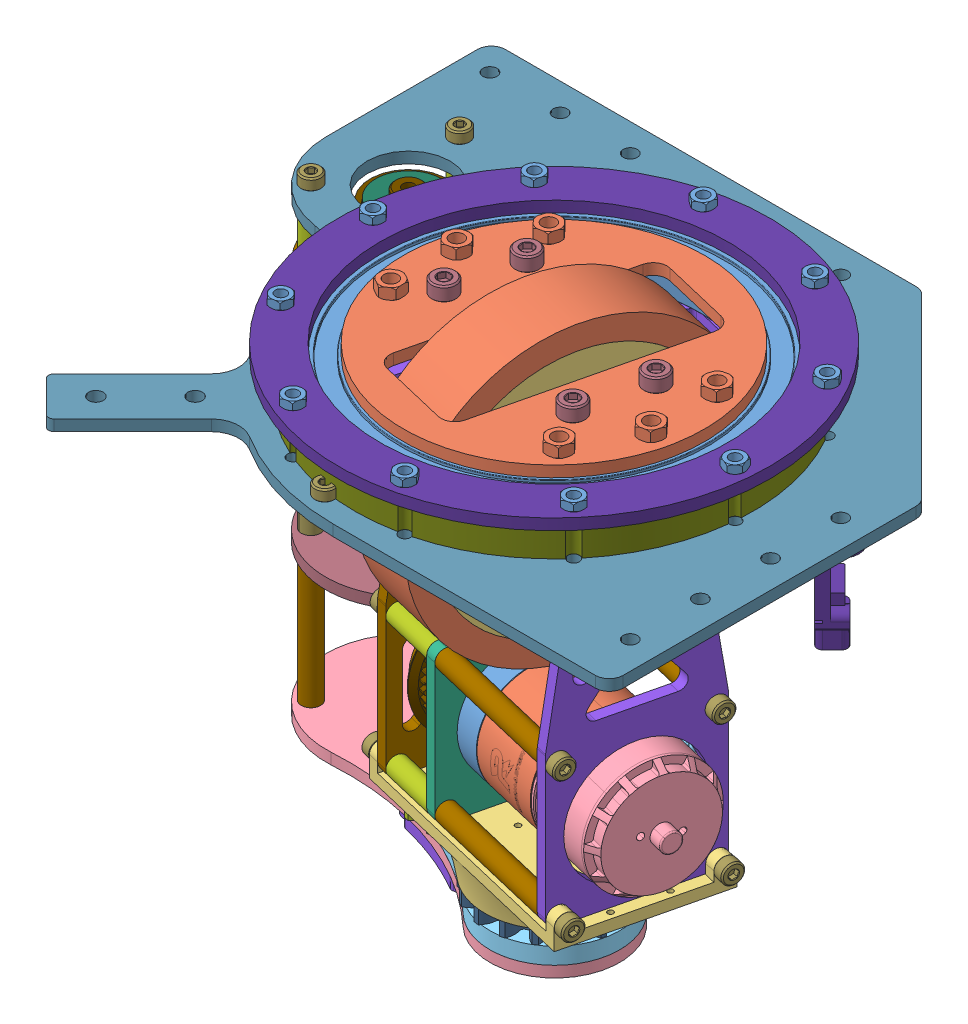
SolidWorks assembly 舵轮装配3508转向板R, configuration 默认. Lengths in mm.
Overall size (849.08 223.15 204.82).
168 component instances, 59 part files, 248 mates.
Components (placement in the parent):
- am-0198 4in Plaction Wheel-1: am-0198 4in Plaction Wheel [默认] at (-7.6128 -124.2866 103.0773) x (0.972741 0 0.231893) z (0.060048 0.965891 -0.25189)
  - am-0198 4in Plaction Wheel(2)^am-0198 4in Plaction Wheel-1: am-0198 4in Plaction Wheel(2)^am-0198 4in Plaction Wheel [默认] at origin (virtual)
- HRB 61821薄圈轴承-1: HRB 61821薄圈轴承 [默认] at (-20.3948 -93.8434 93.3472) x (0.952416 0 0.304802) z (-0.304802 0 0.952416) size (130 13 130)
- 舵轮底板-1: 舵轮底板 [默认] at (-20.3948 -80.8434 93.3472) x (0.231893 0 -0.972741) z (0.972741 0 0.231893) size (109 4 109)
- 舵轮侧面支撑-1: 舵轮侧面支撑 [默认] at (8.3011 -80.8434 100.1881) x (-0.972741 0 -0.231893) z (-0.231893 0 0.972741) size (14 45 35)
- 22 8 7轴承-1: 22 8 7轴承 [默认] at (-15.0447 -115.8434 94.6227) x (-0.972741 0 -0.231893) z (0.221934 -0.28991 -0.930966) size (7 25 25)
- 舵轮用钢轴-1: 舵轮用钢轴 [默认] at (13.1648 -115.8434 101.3476) x (-0.0855 0.929546 0.358656) z (-0.215555 -0.368706 0.904208) size (8 70 8)
- 舵轮侧面支撑B-1: 舵轮侧面支撑B [默认] at (-52.9816 -80.8434 85.5788) x (0.972741 0 0.231893) z (0.231893 0 -0.972741) size (8 45 35)
- 舵轮轴承契合垫-1: 舵轮轴承契合垫 [默认] at (-20.3948 -93.8434 93.3472) x (-0.972741 0 -0.231893) z (0.231893 0 -0.972741) size (18.69 13 65.65)
- 舵轮上底板-1: 舵轮上底板 [默认] at (-20.3948 -97.8434 93.3472) x (0.231893 0 -0.972741) z (0.972741 0 0.231893) size (120 4 120)
- M3508电机安装板-1: M3508电机安装板 [默认] at (-56.8726 -93.3434 84.6513) x (0 1 0) z (-0.231893 0 0.972741) size (145.98 4 55)
- RoboMaster M3508直流无刷减速电-1: RoboMaster M3508直流无刷减速电 [默认] at (54.6807 -194.7601 92.9675) x (0.079289 -0.939729 -0.332601) z (-0.972741 0 -0.231893) size (77.46 77.46 98.4)
  - RoboMaster M3508直流无刷减速电 (1).STEP-1: RoboMaster M3508直流无刷减速电 (1).STEP [默认] at origin size (77.46 77.46 98.4)
    - 4_ASM_1.STEP-1: 4_ASM_1.STEP [默认] at (-1.7887 18.2683 39.841) x (-0.923508 0.383579 0) z (0.383579 0.923508 0) size (13.16 4.26 21.29)
      - __-__10_1__1.STEP-1: __-__10_1__1.STEP [默认] at origin size (2.4 2.3 2.24)
      - __-__10_3__1.STEP-1: __-__10_3__1.STEP [默认] at origin size (2.4 2.3 2.24)
      - __-__10_2__1.STEP-1: __-__10_2__1.STEP [默认] at origin size (2.4 2.3 2.24)
      - __-__20_1.STEP-1: __-__20_1.STEP [默认] at origin size (5.92 4.26 12.18)
    - 2_ASM.STEP-1: 2_ASM.STEP [默认] at (-1.7887 18.2683 50.441) x (-0.378508 0.925598 0) z (0.925598 0.378508 0) size (59.4 67.29 59.4)
      - 26_ASM.STEP-1: 26_ASM.STEP [默认] at (0 34.5 0) x (-0.381788 0 0.92425) z (-0.92425 0 -0.381788) size (22 6 22)
        - 28_1.STEP-1: 28_1.STEP [默认] at (0 2.5 0) size (20 0.2 20)
        - 27_1.STEP-1: 27_1.STEP [默认] at origin size (22 6 22)
        - 28_1.STEP-2: 28_1.STEP [默认] at (0 -2.7 0) size (20 0.2 20)
      - 26_ASM-1.STEP-1: 26_ASM-1.STEP [默认] at (0 27 0) x (-0.381788 0 0.92425) z (-0.92425 0 -0.381788) size (22 6 22)
        - 28_1.STEP-1: 28_1.STEP [默认] at (0 2.5 0) size (20 0.2 20)
        - 27_1.STEP-1: 27_1.STEP [默认] at origin size (22 6 22)
        - 28_1.STEP-2: 28_1.STEP [默认] at (0 -2.7 0) size (20 0.2 20)
      - 25_1.STEP-1: 25_1.STEP [默认] at (0 38.5 0) x (0 0 1) z (-1 0 0) size (16.7 1 13.43)
      - 18_1.STEP-1: 18_1.STEP [默认] at (-12.3744 22 -12.3744) x (0.381788 0 -0.92425) z (0.92425 0 0.381788) size (5.5 37.99 5.5)
      - 17_1.STEP-1: 17_1.STEP [默认] at (0 19.3 0) x (-1 0 0) z (0 0 -1) size (26 44 26)
      - 16_1.STEP-1: 16_1.STEP [默认] at (0 31 0) x (-0.707107 0 0.707107) z (0 1 0) size (42 42 14)
      - 18_1.STEP-2: 18_1.STEP [默认] at (12.3744 22 -12.3744) x (0.92425 0 0.381788) z (-0.381788 0 0.92425) size (5.5 37.99 5.5)
      - 23_1.STEP-1: 23_1.STEP [默认] at origin size (42.11 26 42)
      - 18_1.STEP-3: 18_1.STEP [默认] at (12.3744 22 12.3744) x (-0.381788 0 0.92425) z (-0.92425 0 -0.381788) size (5.5 37.99 5.5)
      - 18_1.STEP-4: 18_1.STEP [默认] at (-12.3744 22 12.3744) x (-0.92425 0 -0.381788) z (0.381788 0 -0.92425) size (5.5 37.99 5.5)
      - 24_1.STEP-1: 24_1.STEP [默认] at (0 37.71 0) x (0 1 0) z (0.381788 0 -0.92425) size (0.42 16 16)
    - 1_1_1.STEP-1: 1_1_1.STEP [默认] at (-1.7887 18.2683 48.441) x (0.923508 -0.383579 0) z (0 0 1) size (42 42 43.4)
    - 3_1.STEP-1: 3_1.STEP [默认] at (4.5067 -1.7659 43.091) x (0.299781 -0.954008 0) z (0.954008 0.299781 0) size (5.77 4 14.5)
- M3508电机安装延长-1: M3508电机安装延长 [默认] at (-37.4178 -199.3254 89.2891) x (0 1 0) z (0.231893 0 -0.972741) size (55 4 55)
- 螺纹M4_长度20铝柱-1: 螺纹M4_长度20铝柱 [默认] at (-42.9832 -223.3254 112.6349) x (0.178665 -0.637485 -0.749461) z (0.147828 0.770463 -0.620108) size (7 20 7)
- 螺纹M4_长度20铝柱-2: 螺纹M4_长度20铝柱 [默认] at (-31.8523 -223.3254 65.9433) x (0.178665 -0.637485 -0.749461) z (0.147828 0.770463 -0.620108) size (7 20 7)
- 螺纹M4_长度20铝柱-3: 螺纹M4_长度20铝柱 [默认] at (-42.9832 -175.3254 112.6349) x (0.178665 -0.637485 -0.749461) z (0.147828 0.770463 -0.620108) size (7 20 7)
- 螺纹M4_长度20铝柱-4: 螺纹M4_长度20铝柱 [默认] at (-31.8523 -175.3254 65.9433) x (0.178665 -0.637485 -0.749461) z (0.147828 0.770463 -0.620108) size (7 20 7)
- M3508电机安装板B-1: M3508电机安装板B [默认] at (19.0012 -93.3434 102.7389) x (0 1 0) z (-0.231893 0 0.972741) size (145.98 4 55)
- 螺纹M4_长度50铝柱-1: 螺纹M4_长度50铝柱 [默认] at (20.6757 -175.3254 78.4655) x (0.131851 -0.822624 -0.553086) z (0.190761 0.568585 -0.800201) size (7 50 7)
- 螺纹M4_长度50铝柱-2: 螺纹M4_长度50铝柱 [默认] at (20.6757 -223.3254 78.4655) x (0.131851 -0.822624 -0.553086) z (0.190761 0.568585 -0.800201) size (7 50 7)
- 螺纹M4_长度50铝柱-3: 螺纹M4_长度50铝柱 [默认] at (9.5448 -223.3254 125.1571) x (0.131851 -0.822624 -0.553086) z (0.190761 0.568585 -0.800201) size (7 50 7)
- 螺纹M4_长度50铝柱-4: 螺纹M4_长度50铝柱 [默认] at (9.5448 -175.3254 125.1571) x (0.131851 -0.822624 -0.553086) z (0.190761 0.568585 -0.800201) size (7 50 7)
- 舵轮用100齿3m同步带-1: 舵轮用100齿3m同步带 [默认] at (-39.6585 -199.3254 88.7549) x (-0.00142 0.999981 0.005957) z (-0.231889 -0.006124 0.972723) size (119.08 7 42.19)
- 舵轮轴承契合垫B-1: 舵轮轴承契合垫B [默认] at (-20.3948 -93.8434 93.3472) x (0.972741 0 0.231893) z (-0.231893 0 0.972741) size (18.69 13 65.65)
- M4螺丝头-3: M4螺丝头 [默认] at (-66.329 -175.3254 107.0695) x (0.075861 -0.944977 -0.31822) z (0.219133 0.327137 -0.919218) size (7.2 4.15 7.2)
- M4螺丝头-4: M4螺丝头 [默认] at (-55.1981 -175.3254 60.3779) x (0.077323 -0.94277 -0.324353) z (0.218622 0.333443 -0.917072) size (7.2 4.15 7.2)
- M4螺丝头-6: M4螺丝头 [默认] at (24.5667 -175.3254 79.3931) x (0.143947 0.784011 -0.603826) z (0.181807 -0.620747 -0.76264) size (7.2 4.15 7.2)
- M4螺丝头-7: M4螺丝头 [默认] at (13.4358 -175.3254 126.0847) x (0.143947 0.784011 -0.603826) z (0.181807 -0.620747 -0.76264) size (7.2 4.15 7.2)
- M5螺丝头-1: M5螺丝头 [默认] at (17.8418 -85.8434 107.6026) x (0.144633 0.781658 -0.606706) z (0.181261 -0.623708 -0.760351) size (8.7 5.42 8.7)
- M5螺丝头-2: M5螺丝头 [默认] at (20.1607 -85.8434 97.8752) x (0.144633 0.781658 -0.606706) z (0.181261 -0.623708 -0.760351) size (8.7 5.42 8.7)
- M5螺丝头-3: M5螺丝头 [默认] at (21.3202 -100.8434 93.0115) x (0.143947 0.784011 -0.603826) z (0.181807 -0.620747 -0.76264) size (8.7 5.42 8.7)
- M5螺丝头-4: M5螺丝头 [默认] at (16.6823 -100.8434 112.4663) x (0.143947 0.784011 -0.603826) z (0.181807 -0.620747 -0.76264) size (8.7 5.42 8.7)
- 舵轮转向同步轮 75齿-3: 舵轮转向同步轮 75齿 [默认] at (-20.4563 -110.3434 93.5041) x (0.231893 0 -0.972741) z (0 1 0) size (120.22 120.22 12.5)
- 螺纹M4_长度20铝柱-5: 螺纹M4_长度20铝柱 [默认] at (-118.8835 -117.8434 29.0349) x (0.334336 0 -0.942454) z (0.942454 0 0.334336) size (7 20 7)
- 螺纹M4_长度20铝柱-6: 螺纹M4_长度20铝柱 [默认] at (-131.2035 -117.8434 70.5466) x (0.991825 0 0.127608) z (-0.127608 0 0.991825) size (7 20 7)
- 螺纹M4_长度20铝柱-7: 螺纹M4_长度20铝柱 [默认] at (-89.0934 -117.8434 60.4602) x (0.952416 0 0.304802) z (-0.304802 0 0.952416) size (7 20 7)
- 舵轮转向驱动同步轮15齿-1: 舵轮转向驱动同步轮15齿 [默认] at (-113.0601 -108.8434 53.3472) x (0.894911 0 0.446244) z (0 1 0) size (23.73 23.73 12)
- M5螺丝头-7: M5螺丝头 [默认] at (25.1276 -105.3434 79.7838) x (-0.621955 0 -0.783053) z (-0.783053 0 0.621955) size (8.7 5.42 8.7)
- M5螺丝头-8: M5螺丝头 [默认] at (25.8104 -105.3434 104.3622) x (-0.598714 0 -0.800963) z (-0.800963 0 0.598714) size (8.7 5.42 8.7)
- M5螺丝头-9: M5螺丝头 [默认] at (14.1126 -105.3434 125.989) x (-0.602334 0 -0.798244) z (-0.798244 0 0.602334) size (8.7 5.42 8.7)
- M5螺丝头-10: M5螺丝头 [默认] at (-54.9022 -105.3434 60.7054) x (-0.578379 0 -0.815768) z (-0.815768 0 0.578379) size (8.7 5.42 8.7)
- M5螺丝头-11: M5螺丝头 [默认] at (-66.6 -105.3434 82.3323) x (-0.630623 0 -0.776089) z (-0.776089 0 0.630623) size (8.7 5.42 8.7)
- M5螺丝头-12: M5螺丝头 [默认] at (-58.4446 -100.8434 73.9963) x (0.084545 -0.931169 -0.35465) z (0.215931 0.364588 -0.905786) size (8.7 5.42 8.7)
- M5螺丝头-13: M5螺丝头 [默认] at (-65.9171 -105.3434 106.9107) x (-0.636639 0 -0.771162) z (-0.771162 0 0.636639) size (8.7 5.42 8.7)
- M5螺丝头-14: M5螺丝头 [默认] at (-63.0825 -100.8434 93.4511) x (0.110669 -0.878771 -0.464234) z (0.203781 0.477243 -0.854817) size (8.7 5.42 8.7)
- 舵轮大轴承定位环-1: 舵轮大轴承定位环 [默认] at (-20.3948 -93.8434 93.3472) x (0.224951 0 0.97437) z (-0.97437 0 0.224951) size (144.14 13 144.2)
- 轴承压住-1: 轴承压住 [默认] at (-20.3948 -80.8434 93.3472) x (-0.390731 0 0.920505) z (-0.920505 0 -0.390731) size (156 4 156)
- 舵轮转向同步带90齿5m-1: 舵轮转向同步带90齿5m [默认] at (-113.0601 -108.8434 53.3472) x (-0.394392 0 0.918942) z (-0.918942 0 -0.394392) size (124.22 10 176.93)
- M4螺丝头-15: M4螺丝头 [默认] at (-74.8093 -97.8434 46.0454) x (-0.630623 0 -0.776089) z (-0.776089 0 0.630623) size (7.2 4.15 7.2)
- M4螺丝头-16: M4螺丝头 [默认] at (-36.6138 -97.8434 23.0952) x (-0.630623 0 -0.776089) z (-0.776089 0 0.630623) size (7.2 4.15 7.2)
- M4螺丝头-17: M4螺丝头 [默认] at (7.7769 -97.8434 26.9788) x (-0.630623 0 -0.776089) z (-0.776089 0 0.630623) size (7.2 4.15 7.2)
- M4螺丝头-18: M4螺丝头 [默认] at (41.407 -97.8434 56.213) x (-0.630623 0 -0.776089) z (-0.776089 0 0.630623) size (7.2 4.15 7.2)
- M4螺丝头-19: M4螺丝头 [默认] at (51.4309 -97.8434 99.6312) x (-0.630623 0 -0.776089) z (-0.776089 0 0.630623) size (7.2 4.15 7.2)
- M4螺丝头-20: M4螺丝头 [默认] at (34.0198 -97.8434 140.6491) x (-0.630623 0 -0.776089) z (-0.776089 0 0.630623) size (7.2 4.15 7.2)
- M4螺丝头-21: M4螺丝头 [默认] at (-4.1758 -97.8434 163.5993) x (-0.630623 0 -0.776089) z (-0.776089 0 0.630623) size (7.2 4.15 7.2)
- M4螺丝头-22: M4螺丝头 [默认] at (-48.5665 -97.8434 159.7156) x (-0.630623 0 -0.776089) z (-0.776089 0 0.630623) size (7.2 4.15 7.2)
- M4螺丝头-23: M4螺丝头 [默认] at (-82.1965 -97.8434 130.4815) x (-0.630623 0 -0.776089) z (-0.776089 0 0.630623) size (7.2 4.15 7.2)
- M4螺丝头-24: M4螺丝头 [默认] at (-92.2204 -97.8434 87.0633) x (-0.630623 0 -0.776089) z (-0.776089 0 0.630623) size (7.2 4.15 7.2)
- M4螺母-1: M4螺母 [默认] at (51.4309 -76.8434 99.6312) x (0.695285 0 0.718734) z (-0.718734 0 0.695285) size (6.78 3.05 7.83)
- M4螺母-3: M4螺母 [默认] at (-4.1758 -76.8434 163.5993) x (0.912983 0 0.407998) z (-0.407998 0 0.912983) size (6.78 3.05 7.83)
- M4螺母-4: M4螺母 [默认] at (-48.5665 -76.8434 159.7156) x (0.955617 0 0.294613) z (-0.294613 0 0.955617) size (6.78 3.05 7.83)
- M4螺母-5: M4螺母 [默认] at (-82.1965 -76.8434 130.4815) x (0.953713 0 0.300718) z (-0.300718 0 0.953713) size (6.78 3.05 7.83)
- M4螺母-6: M4螺母 [默认] at (-92.2204 -76.8434 87.0633) x (0.952416 0 0.304802) z (-0.304802 0 0.952416) size (6.78 3.05 7.83)
- M4螺母-7: M4螺母 [默认] at (-74.8093 -76.8434 46.0454) x (0.952416 0 0.304802) z (-0.304802 0 0.952416) size (6.78 3.05 7.83)
- M4螺母-8: M4螺母 [默认] at (-36.6138 -76.8434 23.0952) x (0.996847 0 0.079344) z (-0.079344 0 0.996847) size (6.78 3.05 7.83)
- M4螺母-9: M4螺母 [默认] at (7.7769 -76.8434 26.9788) x (0.952416 0 0.304802) z (-0.304802 0 0.952416) size (6.78 3.05 7.83)
- M4螺母-10: M4螺母 [默认] at (41.407 -76.8434 56.213) x (0.897027 0 0.441976) z (-0.441976 0 0.897027) size (6.78 3.05 7.83)
- M4螺母-11: M4螺母 [默认] at (34.0198 -76.8434 140.6491) x (0.965082 0 0.261948) z (-0.261948 0 0.965082) size (6.78 3.05 7.83)
- M5螺丝头-15: M5螺丝头 [默认] at (-50.083 -76.8434 73.4196) x (0.952416 0 0.304802) z (-0.304802 0 0.952416) size (8.7 5.42 8.7)
- M5螺丝头-16: M5螺丝头 [默认] at (-55.8803 -76.8434 97.7381) size (8.7 5.42 8.7)
- M5螺丝头-17: M5螺丝头 [默认] at (5.4024 -76.8434 112.3474) x (0.952416 0 0.304802) z (-0.304802 0 0.952416) size (8.7 5.42 8.7)
- M5螺丝头-18: M5螺丝头 [默认] at (11.1997 -76.8434 88.0288) x (0.952416 0 0.304802) z (-0.304802 0 0.952416) size (8.7 5.42 8.7)
- M4螺丝头-25: M4螺丝头 [默认] at (-131.2035 -93.8434 70.5466) x (0.95084 0 0.309681) z (-0.309681 0 0.95084) size (7.2 4.15 7.2)
- M4螺丝头-26: M4螺丝头 [默认] at (-118.8835 -93.8434 29.0349) x (0.952251 0 0.305316) z (-0.305316 0 0.952251) size (7.2 4.15 7.2)
- M4螺丝头-27: M4螺丝头 [默认] at (-31.1775 -93.8434 165.6069) x (0.999978 0 -0.006592) z (0.006592 0 0.999978) size (7.2 4.15 7.2)
- M5螺母-1: M5螺母 [默认] at (14.1126 -76.8434 125.989) x (0.952416 0 0.304802) z (-0.304802 0 0.952416) size (8 4 9.24)
- M5螺母-2: M5螺母 [默认] at (25.8104 -76.8434 104.3622) x (0.952416 0 0.304802) z (-0.304802 0 0.952416) size (8 4 9.24)
- M5螺母-3: M5螺母 [默认] at (25.1276 -76.8434 79.7838) x (0.952416 0 0.304802) z (-0.304802 0 0.952416) size (8 4 9.24)
- M5螺母-4: M5螺母 [默认] at (-54.9022 -76.8434 60.7054) x (0.952416 0 0.304802) z (-0.304802 0 0.952416) size (8 4 9.24)
- M5螺母-5: M5螺母 [默认] at (-66.6 -76.8434 82.3323) x (0.952416 0 0.304802) z (-0.304802 0 0.952416) size (8 4 9.24)
- M5螺母-6: M5螺母 [默认] at (-65.9171 -76.8434 106.9107) x (0.999422 0 -0.034008) z (0.034008 0 0.999422) size (8 4 9.24)
- 舵轮线引导和角度定位3D打印件-1: 舵轮线引导和角度定位3D打印件 [默认] at (-20.7352 -226.8254 93.2661) x (0.231893 0 -0.972741) z (-0.972741 0 -0.231893) size (73.09 24 90.3)
- 理线和舵轮角度定位支撑-1: 理线和舵轮角度定位支撑 [默认] at (-113.0601 -259.8434 53.3472) x (-0.393621 0 0.919273) z (-0.919273 0 -0.393621) size (60 4 154.24)
- 舵轮角度定位第二齿轮轴承锁定-1: 舵轮角度定位第二齿轮轴承锁定 [默认] at (-61.8199 -249.8434 75.2877) x (-0.919273 0 -0.393621) z (0.393621 0 -0.919273) size (93.42 10.62 47)
- 6704zz轴承-1: 6704zz轴承 [默认] at (-61.8199 -253.8434 75.2877) x (0.929857 0 0.36792) z (-0.36792 0 0.929857) size (27 4 27)
- 舵轮角度定位第二齿轮-1: 舵轮角度定位第二齿轮 [默认] at (-61.8199 -247.3434 75.2877) x (0.291333 0 0.956622) z (0 1 0) size (50.24 50.45 15.5)
- M4螺丝头-28: M4螺丝头 [默认] at (-89.0934 -259.8434 60.4602) x (-0.60814 0 -0.79383) z (-0.79383 0 0.60814) size (7.2 4.15 7.2)
- M4螺丝头-30: M4螺丝头 [默认] at (-131.2035 -259.8434 70.5466) x (-0.602759 0 -0.797923) z (-0.797923 0 0.602759) size (7.2 4.15 7.2)
- M4螺丝头-31: M4螺丝头 [默认] at (17.6186 -223.3254 127.0818) x (0.163039 -0.711114 -0.683912) z (-0.164902 -0.703077 0.69173) size (7.2 4.15 7.2)
- M4螺丝头-32: M4螺丝头 [默认] at (-59.0891 -223.3254 59.4503) x (-0.195604 -0.537113 0.820517) z (0.124553 -0.84351 -0.522472) size (7.2 4.15 7.2)
- M4螺丝头-33: M4螺丝头 [默认] at (-70.2199 -223.3254 106.1419) x (0.230329 0.115959 -0.966179) z (-0.02689 0.993254 0.112798) size (7.2 4.15 7.2)
- M4螺丝头-34: M4螺丝头 [默认] at (28.7495 -223.3254 80.3903) x (0.163039 -0.711114 -0.683912) z (-0.164902 -0.703077 0.69173) size (7.2 4.15 7.2)
- 舵轮角度定位AS5600支撑-1: 舵轮角度定位AS5600支撑 [默认] at (-61.8199 -259.8434 75.2877) x (-0.919273 0 -0.393621) z (0.393621 0 -0.919273) size (49.84 4 35.05)
- 舵轮转向电机安装件M3508版本-1: 舵轮转向电机安装件M3508版本 [默认] at (-113.0601 -121.8434 53.3472) x (-0.284517 0 0.958671) z (-0.958671 0 -0.284517) size (60 4 60)
- RoboMaster M3508直流无刷减速电-2: RoboMaster M3508直流无刷减速电 [默认] at (-121.3423 -208.2844 36.9663) x (-0.932142 0 0.362092) z (0 1 0) size (77.46 77.46 98.4)
  - RoboMaster M3508直流无刷减速电 (1).STEP-1: RoboMaster M3508直流无刷减速电 (1).STEP [默认] at origin size (77.46 77.46 98.4)
    - 4_ASM_1.STEP-1: 4_ASM_1.STEP [默认] at (-1.7887 18.2683 39.841) x (-0.923508 0.383579 0) z (0.383579 0.923508 0) size (13.16 4.26 21.29)
      - __-__10_1__1.STEP-1: __-__10_1__1.STEP [默认] at origin size (2.4 2.3 2.24)
      - __-__10_3__1.STEP-1: __-__10_3__1.STEP [默认] at origin size (2.4 2.3 2.24)
      - __-__10_2__1.STEP-1: __-__10_2__1.STEP [默认] at origin size (2.4 2.3 2.24)
      - __-__20_1.STEP-1: __-__20_1.STEP [默认] at origin size (5.92 4.26 12.18)
    - 2_ASM.STEP-1: 2_ASM.STEP [默认] at (-1.7887 18.2683 50.441) x (-0.378508 0.925598 0) z (0.925598 0.378508 0) size (59.4 67.29 59.4)
      - 26_ASM.STEP-1: 26_ASM.STEP [默认] at (0 34.5 0) x (-0.381788 0 0.92425) z (-0.92425 0 -0.381788) size (22 6 22)
        - 28_1.STEP-1: 28_1.STEP [默认] at (0 2.5 0) size (20 0.2 20)
        - 27_1.STEP-1: 27_1.STEP [默认] at origin size (22 6 22)
        - 28_1.STEP-2: 28_1.STEP [默认] at (0 -2.7 0) size (20 0.2 20)
      - 26_ASM-1.STEP-1: 26_ASM-1.STEP [默认] at (0 27 0) x (-0.381788 0 0.92425) z (-0.92425 0 -0.381788) size (22 6 22)
        - 28_1.STEP-1: 28_1.STEP [默认] at (0 2.5 0) size (20 0.2 20)
        - 27_1.STEP-1: 27_1.STEP [默认] at origin size (22 6 22)
        - 28_1.STEP-2: 28_1.STEP [默认] at (0 -2.7 0) size (20 0.2 20)
      - 25_1.STEP-1: 25_1.STEP [默认] at (0 38.5 0) x (0 0 1) z (-1 0 0) size (16.7 1 13.43)
      - 18_1.STEP-1: 18_1.STEP [默认] at (-12.3744 22 -12.3744) x (0.381788 0 -0.92425) z (0.92425 0 0.381788) size (5.5 37.99 5.5)
      - 17_1.STEP-1: 17_1.STEP [默认] at (0 19.3 0) x (-1 0 0) z (0 0 -1) size (26 44 26)
      - 16_1.STEP-1: 16_1.STEP [默认] at (0 31 0) x (-0.707107 0 0.707107) z (0 1 0) size (42 42 14)
      - 18_1.STEP-2: 18_1.STEP [默认] at (12.3744 22 -12.3744) x (0.92425 0 0.381788) z (-0.381788 0 0.92425) size (5.5 37.99 5.5)
      - 23_1.STEP-1: 23_1.STEP [默认] at origin size (42.11 26 42)
      - 18_1.STEP-3: 18_1.STEP [默认] at (12.3744 22 12.3744) x (-0.381788 0 0.92425) z (-0.92425 0 -0.381788) size (5.5 37.99 5.5)
      - 18_1.STEP-4: 18_1.STEP [默认] at (-12.3744 22 12.3744) x (-0.92425 0 -0.381788) z (0.381788 0 -0.92425) size (5.5 37.99 5.5)
      - 24_1.STEP-1: 24_1.STEP [默认] at (0 37.71 0) x (0 1 0) z (0.381788 0 -0.92425) size (0.42 16 16)
    - 1_1_1.STEP-1: 1_1_1.STEP [默认] at (-1.7887 18.2683 48.441) x (0.923508 -0.383579 0) z (0 0 1) size (42 42 43.4)
    - 3_1.STEP-1: 3_1.STEP [默认] at (4.5067 -1.7659 43.091) x (0.299781 -0.954008 0) z (0.954008 0.299781 0) size (5.77 4 14.5)
- 舵轮转向齿轮拼接-1: 舵轮转向齿轮拼接 [默认] at (-20.7352 -248.8254 93.2661) x (-0.972741 0 -0.231893) z (0.231893 0 -0.972741) size (49.13 17 49.32)
- 27_20_4轴承-1: 27_20_4轴承 [默认] at (-20.4526 -255.8434 93.0006) x (0.977214 0 0.212256) z (-0.212256 0 0.977214) size (27 4 27)
- 螺纹M4_长度80铝柱-4: 螺纹M4_长度80铝柱 [默认] at (-118.8835 -201.8434 29.0349) x (-0.231145 0 0.972919) z (-0.972919 0 -0.231145) size (7 80 7)
- 螺纹M4_长度80铝柱-5: 螺纹M4_长度80铝柱 [默认] at (-131.2035 -201.8434 70.5466) x (-0.277096 0 0.960842) z (-0.960842 0 -0.277096) size (7 80 7)
- 螺纹M4_长度80铝柱-6: 螺纹M4_长度80铝柱 [默认] at (-89.0934 -201.8434 60.4602) x (0.668866 0 0.743383) z (-0.743383 0 0.668866) size (7 80 7)
- 舵轮转向电机安装件-3: 舵轮转向电机安装件 [默认] at (-113.0601 -205.8434 53.3472) x (-0.284517 0 0.958671) z (-0.958671 0 -0.284517) size (60 4 60)
- 螺纹M4_长度50铝柱-8: 螺纹M4_长度50铝柱 [默认] at (-131.2035 -255.8434 70.5466) x (0.823062 0 0.567952) z (-0.567952 0 0.823062) size (7 50 7)
- 螺纹M4_长度50铝柱-9: 螺纹M4_长度50铝柱 [默认] at (-118.8835 -255.8434 29.0349) x (0.96384 0 0.266482) z (-0.266482 0 0.96384) size (7 50 7)
- 螺纹M4_长度50铝柱-10: 螺纹M4_长度50铝柱 [默认] at (-89.0934 -255.8434 60.4602) x (0.841404 0 -0.540407) z (0.540407 0 0.841404) size (7 50 7)
- 舵轮直角安装架R-1: 舵轮直角安装架R [默认] at (-285.7255 -97.8434 93.3472) size (222.67 4 198.17)
- as5600安装架小-1: as5600安装架小 [默认] at (-61.8199 -261.8434 75.2877) x (0.393621 0 -0.919273) z (-0.919273 0 -0.393621) size (23 3 23)
- 第二齿轮上固定-1: 第二齿轮上固定 [默认] at (-61.8199 -251.8434 75.2877) x (-0.956622 0 0.291333) z (0.291333 0 0.956622) size (22 3.5 22)
- as5600安装架小-2: as5600安装架小 [默认] at (-61.8199 -267.8434 75.2877) x (0.919273 0 0.393621) z (-0.393621 0 0.919273) size (23 3 23)
- 配电板支架R-1: 配电板支架R [默认] at (31.5052 -97.8434 41.4472) x (0 0 -1) z (-1 0 0) size (89.5 55 843.45)
- 40齿3M同步轮-1: 40齿3M同步轮 [GearTrax] at (-50.3552 -199.3254 86.2049) x (0.009093 0.999231 -0.038144) z (0.972741 0 0.231893) size (43.17 43.17 18.61)
- 16_8_5轴承-1: 16_8_5轴承 [默认] at (-27.5931 -115.8434 91.6312) x (0.972741 0 0.231893) z (-0.231392 0.065672 0.970641) size (5 17 17)
- 包胶轮子装配-1: 包胶轮子装配 [默认] at (-7.0413 -25.7462 40.883) x (0.20398 -0.475659 -0.855652) z (-0.110302 -0.87963 0.462693) size (105 25 105)
  - 定制轮子包胶部分-1: 定制轮子包胶部分 [默认] at (-4.7594 -13.3234 105) size (105 25 105)
  - 定制轮子铝合金部分-1: 定制轮子铝合金部分 [默认] at (-4.7594 -13.3234 105) size (88 25 88)
- 包胶轮子同步轮-1: 包胶轮子同步轮 [默认] at (-57.0824 24.1318 171.778) x (0.20398 -0.475659 -0.855652) z (0.972741 0 0.231893) size (63 58.51 16)
- 包胶轮子垫圈-1: 包胶轮子垫圈 [默认] at (1.4919 -115.8434 98.5648) x (-0.074139 0.947515 0.310996) z (-0.219722 -0.319711 0.921687) size (20 10 20)
Mates (geometry in assembly coordinates):
- 同心2: concentric aligned: cylinder of HRB 61821薄圈轴承-1 through (-20.3948 -80.8434 93.3472) axis (0 -1 0) radius 65; cylinder of 舵轮底板-1 through (-20.3948 -76.8434 93.3472) axis (0 -1 0) radius 54.5
- 平行1: parallel anti-aligned: plane of am-0198 4in Plaction Wheel-1/am-0198 4in Plaction Wheel(2)^am-0198 4in Plaction Wheel-1/4 Modular Half^am-0198 4in Plaction Wheel(2)_am-0198 4in Plaction Wheel-1 through (-41.2853 -84.2812 91.9114) normal (-0.972741 0 -0.231893); plane of 舵轮底板-1 through (-47.2732 -80.8434 130.6306) normal (0.972741 0 0.231893)
- 重合3: coincident anti-aligned: plane of HRB 61821薄圈轴承-1 through (-20.3948 -80.8434 93.3472) normal (0 1 0); plane of 舵轮底板-1 through (-20.3948 -80.8434 93.3472) normal (0 -1 0)
- 同心3: concentric anti-aligned: cylinder of 舵轮底板-1 through (11.1997 -70.8434 88.0288) axis (0 -1 0) radius 2.6; cylinder of 舵轮侧面支撑-1 through (11.1997 -90.8434 88.0288) axis (0 1 0) radius 2.1
- 重合4: coincident anti-aligned: plane of 舵轮底板-1 through (-20.3948 -80.8434 93.3472) normal (0 -1 0); plane of 舵轮侧面支撑-1 through (8.3011 -80.8434 100.1881) normal (0 1 0)
- 同心5: concentric anti-aligned: cylinder of 舵轮底板-1 through (5.4024 -70.8434 112.3474) axis (0 -1 0) radius 2.6; cylinder of 舵轮侧面支撑-1 through (5.4024 -90.8434 112.3474) axis (0 1 0) radius 2.1
- 同心6: concentric aligned: cone of am-0198 4in Plaction Wheel-1/am-0198 4in Plaction Wheel(2)^am-0198 4in Plaction Wheel-1/4 Modular Half^am-0198 4in Plaction Wheel(2)_am-0198 4in Plaction Wheel-2 through (0.0347 -115.8434 98.2175) axis (-0.972741 0 -0.231893); cylinder of 舵轮侧面支撑-1 through (46.238 -115.8434 109.2319) axis (-0.972741 0 -0.231893) radius 4.05
- 同心12: concentric anti-aligned: cylinder of 舵轮侧面支撑-1 through (46.238 -115.8434 109.2319) axis (-0.972741 0 -0.231893) radius 4.05; cylinder of 舵轮用钢轴-1 through (-54.9271 -115.8434 85.1151) axis (0.972741 0 0.231893) radius 4
- 重合12: coincident aligned: plane of 舵轮侧面支撑-1 through (13.1648 -115.8434 101.3476) normal (-0.972741 0 -0.231893); circle of 舵轮用钢轴-1
- 同心13: concentric aligned: cylinder of 舵轮用钢轴-1 through (-54.9271 -115.8434 85.1151) axis (0.972741 0 0.231893) radius 4; cylinder of 舵轮侧面支撑B-1 through (-93.8368 -115.8434 75.8393) axis (0.972741 0 0.231893) radius 4.05
- 同心14: concentric anti-aligned: cylinder of 舵轮侧面支撑B-1 through (-50.083 -90.8434 73.4196) axis (0 1 0) radius 2.1; cylinder of 舵轮底板-1 through (-50.083 19.1566 73.4196) axis (0 -1 0) radius 2.6
- 同心15: concentric aligned: cylinder of 舵轮底板-1 through (25.8104 -70.8434 104.3622) axis (0 -1 0) radius 2.6; cylinder of 舵轮轴承契合垫-1 through (25.8104 -80.8434 104.3622) axis (0 -1 0) radius 2.6
- 同心16: concentric aligned: cylinder of 舵轮底板-1 through (25.1276 -70.8434 79.7838) axis (0 -1 0) radius 2.6; cylinder of 舵轮轴承契合垫-1 through (25.1276 -80.8434 79.7838) axis (0 -1 0) radius 2.6
- 重合14: coincident anti-aligned: plane of 舵轮轴承契合垫-1 through (-20.3948 -80.8434 93.3472) normal (0 1 0); plane of 舵轮底板-1 through (-20.3948 -80.8434 93.3472) normal (0 -1 0)
- 同心19: concentric aligned: cylinder of HRB 61821薄圈轴承-1 through (-20.3948 -80.8434 93.3472) axis (0 -1 0) radius 65; cylinder of 舵轮上底板-1 through (-20.3948 75.8622 93.3472) axis (0 -1 0) radius 60
- 重合16: coincident anti-aligned: plane of HRB 61821薄圈轴承-1 through (-20.3948 -93.8434 93.3472) normal (0 -1 0); plane of 舵轮上底板-1 through (-20.3948 -93.8434 93.3472) normal (0 1 0)
- 同心21: concentric anti-aligned: cylinder of 舵轮侧面支撑-1 through (99.9255 -85.8434 116.8904) axis (-0.972741 0 -0.231893) radius 2.1; cylinder of M3508电机安装板-1 through (-59.6041 -85.8434 78.86) axis (0.972741 0 0.231893) radius 2.6
- 同心22: concentric anti-aligned: cylinder of 舵轮侧面支撑-1 through (101.085 -100.8434 112.0267) axis (-0.972741 0 -0.231893) radius 2.1; cylinder of M3508电机安装板-1 through (-58.4446 -100.8434 73.9963) axis (0.972741 0 0.231893) radius 2.6
- 重合17: coincident anti-aligned: plane of 舵轮侧面支撑B-1 through (-56.8726 -115.8434 84.6513) normal (-0.972741 0 -0.231893); plane of M3508电机安装板-1 through (-56.8726 -93.3434 84.6513) normal (0.972741 0 0.231893)
- 同心23: concentric anti-aligned: cylinder of M3508电机安装板-1 through (-51.0361 -199.3254 86.0426) axis (-0.972741 0 -0.231893) radius 13.15; circle of RoboMaster M3508直流无刷减速电-1/2_ASM-1/16_1-1
- 同心24: concentric anti-aligned: cylinder of M3508电机安装板-1 through (-45.4707 -175.3254 62.6968) axis (-0.972741 0 -0.231893) radius 2.1; cylinder of M3508电机安装延长-1 through (-31.8523 -175.3254 65.9433) axis (0.972741 0 0.231893) radius 2.1
- 同心25: concentric anti-aligned: cylinder of M3508电机安装板-1 through (-51.0361 -199.3254 86.0426) axis (-0.972741 0 -0.231893) radius 13.15; cylinder of M3508电机安装延长-1 through (-37.4178 -199.3254 89.2891) axis (0.972741 0 0.231893) radius 13.15
- 重合18: coincident anti-aligned: plane of RoboMaster M3508直流无刷减速电-1/2_ASM-1/16_1-1 through (-31.3132 -190.5006 80.9311) normal (-0.972741 0 -0.231893); plane of M3508电机安装延长-1 through (-33.5268 -199.3254 90.2167) normal (0.972741 0 0.231893)
- 同心27: concentric anti-aligned: cylinder of M3508电机安装板-1 through (-56.6016 -223.3254 109.3884) axis (-0.972741 0 -0.231893) radius 2.1; cylinder of 螺纹M4_长度20铝柱-1 through (-62.438 -223.3254 107.9971) axis (0.972741 0 0.231893) radius 3.5
- 重合19: coincident anti-aligned: plane of M3508电机安装板-1 through (-56.8726 -93.3434 84.6513) normal (0.972741 0 0.231893); plane of 螺纹M4_长度20铝柱-1 through (-62.438 -223.3254 107.9971) normal (-0.972741 0 -0.231893)
- 重合20: coincident anti-aligned: plane of M3508电机安装延长-1 through (-37.4178 -199.3254 89.2891) normal (-0.972741 0 -0.231893); plane of 螺纹M4_长度20铝柱-1 through (-42.9832 -223.3254 112.6349) normal (0.972741 0 0.231893)
- 同心29: concentric anti-aligned: cylinder of M3508电机安装板-1 through (-56.6016 -175.3254 109.3884) axis (-0.972741 0 -0.231893) radius 2.1; cylinder of 螺纹M4_长度20铝柱-3 through (-62.438 -175.3254 107.9971) axis (0.972741 0 0.231893) radius 3.5
- 同心30: concentric anti-aligned: cylinder of M3508电机安装板-1 through (-45.4707 -175.3254 62.6968) axis (-0.972741 0 -0.231893) radius 2.1; cylinder of 螺纹M4_长度20铝柱-4 through (-51.3072 -175.3254 61.3055) axis (0.972741 0 0.231893) radius 3.5
- 同心31: concentric anti-aligned: cylinder of M3508电机安装板-1 through (-45.4707 -223.3254 62.6968) axis (-0.972741 0 -0.231893) radius 2.1; cylinder of 螺纹M4_长度20铝柱-2 through (-51.3072 -223.3254 61.3055) axis (0.972741 0 0.231893) radius 3.5
- 重合21: coincident anti-aligned: plane of M3508电机安装板-1 through (-56.8726 -93.3434 84.6513) normal (0.972741 0 0.231893); plane of 螺纹M4_长度20铝柱-2 through (-51.3072 -223.3254 61.3055) normal (-0.972741 0 -0.231893)
- 重合22: coincident anti-aligned: plane of M3508电机安装延长-1 through (-37.4178 -199.3254 89.2891) normal (-0.972741 0 -0.231893); plane of 螺纹M4_长度20铝柱-4 through (-31.8523 -175.3254 65.9433) normal (0.972741 0 0.231893)
- 重合23: coincident anti-aligned: plane of M3508电机安装板-1 through (-56.8726 -93.3434 84.6513) normal (0.972741 0 0.231893); plane of 螺纹M4_长度20铝柱-3 through (-62.438 -175.3254 107.9971) normal (-0.972741 0 -0.231893)
- 重合27: coincident anti-aligned: plane of 舵轮侧面支撑-1 through (11.0521 -140.8434 118.8343) normal (0.972741 0 0.231893); plane of M3508电机安装板B-1 through (15.1103 -93.3434 101.8113) normal (-0.972741 0 -0.231893)
- 同心36: concentric anti-aligned: cylinder of 舵轮侧面支撑-1 through (96.4471 -100.8434 131.4815) axis (-0.972741 0 -0.231893) radius 2.1; cylinder of M3508电机安装板B-1 through (12.7913 -100.8434 111.5388) axis (0.972741 0 0.231893) radius 2.6
- 同心37: concentric anti-aligned: cylinder of 舵轮侧面支撑-1 through (101.085 -100.8434 112.0267) axis (-0.972741 0 -0.231893) radius 2.1; cylinder of M3508电机安装板B-1 through (17.4292 -100.8434 92.0839) axis (0.972741 0 0.231893) radius 2.6
- 同心39: concentric anti-aligned: cylinder of M3508电机安装板B-1 through (19.2723 -223.3254 127.4761) axis (-0.972741 0 -0.231893) radius 2.1; cylinder of 螺纹M4_长度50铝柱-3 through (-39.0922 -223.3254 113.5625) axis (0.972741 0 0.231893) radius 3.5
- 同心40: concentric anti-aligned: cylinder of M3508电机安装板B-1 through (30.4031 -223.3254 80.7845) axis (-0.972741 0 -0.231893) radius 2.1; cylinder of 螺纹M4_长度50铝柱-2 through (-27.9614 -223.3254 66.8709) axis (0.972741 0 0.231893) radius 3.5
- 同心41: concentric anti-aligned: cylinder of M3508电机安装板B-1 through (30.4031 -175.3254 80.7845) axis (-0.972741 0 -0.231893) radius 2.1; cylinder of 螺纹M4_长度50铝柱-1 through (-27.9614 -175.3254 66.8709) axis (0.972741 0 0.231893) radius 3.5
- 同心42: concentric anti-aligned: cylinder of M3508电机安装板B-1 through (19.2723 -175.3254 127.4761) axis (-0.972741 0 -0.231893) radius 2.1; cylinder of 螺纹M4_长度50铝柱-4 through (-39.0922 -175.3254 113.5625) axis (0.972741 0 0.231893) radius 3.5
- 重合28: coincident anti-aligned: plane of M3508电机安装板B-1 through (15.1103 -93.3434 101.8113) normal (-0.972741 0 -0.231893); plane of 螺纹M4_长度50铝柱-2 through (20.6757 -223.3254 78.4655) normal (0.972741 0 0.231893)
- 重合29: coincident anti-aligned: plane of M3508电机安装延长-1 through (-33.5268 -199.3254 90.2167) normal (0.972741 0 0.231893); plane of 螺纹M4_长度50铝柱-3 through (-39.0922 -223.3254 113.5625) normal (-0.972741 0 -0.231893)
- 重合30: coincident anti-aligned: plane of M3508电机安装板B-1 through (15.1103 -93.3434 101.8113) normal (-0.972741 0 -0.231893); plane of 螺纹M4_长度50铝柱-1 through (20.6757 -175.3254 78.4655) normal (0.972741 0 0.231893)
- 重合31: coincident anti-aligned: plane of M3508电机安装板B-1 through (15.1103 -93.3434 101.8113) normal (-0.972741 0 -0.231893); plane of 螺纹M4_长度50铝柱-4 through (9.5448 -175.3254 125.1571) normal (0.972741 0 0.231893)
- 同心56: concentric aligned: cylinder of 舵轮底板-1 through (-66.6 -70.8434 82.3323) axis (0 -1 0) radius 2.6; cylinder of 舵轮轴承契合垫B-1 through (-66.6 -80.8434 82.3323) axis (0 -1 0) radius 2.6
- 同心57: concentric aligned: cylinder of 舵轮底板-1 through (-65.9171 -70.8434 106.9107) axis (0 -1 0) radius 2.6; cylinder of 舵轮轴承契合垫B-1 through (-65.9171 -80.8434 106.9107) axis (0 -1 0) radius 2.6
- 重合34: coincident anti-aligned: plane of 舵轮底板-1 through (-20.3948 -80.8434 93.3472) normal (0 -1 0); plane of 舵轮轴承契合垫B-1 through (-20.3948 -80.8434 93.3472) normal (0 1 0)
- 同心59: concentric anti-aligned: cylinder of M4螺丝头-3 through (-70.2199 -175.3254 106.1419) axis (0.972741 0 0.231893) radius 3.6; cylinder of M3508电机安装板-1 through (-56.6016 -175.3254 109.3884) axis (-0.972741 0 -0.231893) radius 2.1
- 同心60: concentric anti-aligned: cylinder of M3508电机安装板-1 through (-45.4707 -175.3254 62.6968) axis (-0.972741 0 -0.231893) radius 2.1; cylinder of M4螺丝头-4 through (-59.0891 -175.3254 59.4503) axis (0.972741 0 0.231893) radius 3.6
- 重合37: coincident anti-aligned: plane of M3508电机安装板-1 through (-60.7636 -93.3434 83.7237) normal (-0.972741 0 -0.231893); plane of M4螺丝头-4 through (-55.1981 -175.3254 60.3779) normal (0.972741 0 0.231893)
- 重合38: coincident anti-aligned: plane of M3508电机安装板-1 through (-60.7636 -93.3434 83.7237) normal (-0.972741 0 -0.231893); plane of M4螺丝头-3 through (-66.329 -175.3254 107.0695) normal (0.972741 0 0.231893)
- 重合41: coincident anti-aligned: plane of M3508电机安装板B-1 through (19.0012 -93.3434 102.7389) normal (0.972741 0 0.231893); plane of M4螺丝头-7 through (13.4358 -175.3254 126.0847) normal (-0.972741 0 -0.231893)
- 同心64: concentric aligned: cylinder of M3508电机安装板B-1 through (19.2723 -175.3254 127.4761) axis (-0.972741 0 -0.231893) radius 2.1; cylinder of M4螺丝头-7 through (17.3268 -175.3254 127.0123) axis (-0.972741 0 -0.231893) radius 3.6
- 重合42: coincident anti-aligned: plane of M3508电机安装板B-1 through (19.0012 -93.3434 102.7389) normal (0.972741 0 0.231893); plane of M4螺丝头-6 through (24.5667 -175.3254 79.3931) normal (-0.972741 0 -0.231893)
- 同心65: concentric aligned: cylinder of M3508电机安装板B-1 through (30.4031 -175.3254 80.7845) axis (-0.972741 0 -0.231893) radius 2.1; cylinder of M4螺丝头-6 through (28.4576 -175.3254 80.3207) axis (-0.972741 0 -0.231893) radius 3.6
- 同心70: concentric anti-aligned: cylinder of M3508电机安装板B-1 through (17.4292 -100.8434 92.0839) axis (0.972741 0 0.231893) radius 2.6; cylinder of M5螺丝头-3 through (26.1839 -100.8434 94.171) axis (-0.972741 0 -0.231893) radius 4.35
- 同心71: concentric anti-aligned: cylinder of M3508电机安装板B-1 through (12.7913 -100.8434 111.5388) axis (0.972741 0 0.231893) radius 2.6; cylinder of M5螺丝头-4 through (21.546 -100.8434 113.6258) axis (-0.972741 0 -0.231893) radius 4.35
- 重合47: coincident anti-aligned: plane of M3508电机安装板B-1 through (19.0012 -93.3434 102.7389) normal (0.972741 0 0.231893); circle of M5螺丝头-4
- 重合48: coincident anti-aligned: plane of M3508电机安装板B-1 through (19.0012 -93.3434 102.7389) normal (0.972741 0 0.231893); plane of M5螺丝头-3 through (21.3202 -100.8434 93.0115) normal (-0.972741 0 -0.231893)
- 同心72: concentric anti-aligned: cylinder of M3508电机安装板B-1 through (16.2697 -85.8434 96.9476) axis (0.972741 0 0.231893) radius 2.6; cylinder of M5螺丝头-2 through (25.0244 -85.8434 99.0347) axis (-0.972741 0 -0.231893) radius 4.35
- 重合49: coincident anti-aligned: plane of M3508电机安装板B-1 through (19.0012 -93.3434 102.7389) normal (0.972741 0 0.231893); plane of M5螺丝头-2 through (20.1607 -85.8434 97.8752) normal (-0.972741 0 -0.231893)
- 重合50: coincident anti-aligned: plane of M3508电机安装板B-1 through (19.0012 -93.3434 102.7389) normal (0.972741 0 0.231893); plane of M5螺丝头-1 through (17.8418 -85.8434 107.6026) normal (-0.972741 0 -0.231893)
- 同心73: concentric anti-aligned: cylinder of M3508电机安装板B-1 through (13.9508 -85.8434 106.675) axis (0.972741 0 0.231893) radius 2.6; cylinder of M5螺丝头-1 through (22.7055 -85.8434 108.7621) axis (-0.972741 0 -0.231893) radius 4.35
- 重合56: coincident anti-aligned: plane of 舵轮上底板-1 through (-20.3948 -97.8434 93.3472) normal (0 -1 0); plane of 舵轮转向同步轮 75齿-3 through (-20.4563 -97.8434 93.5041) normal (0 1 0)
- 同心92: concentric aligned: cylinder of 舵轮上底板-1 through (-54.9022 -87.8434 60.7054) axis (0 -1 0) radius 2.6; cylinder of 舵轮轴承契合垫B-1 through (-54.9022 -80.8434 60.7054) axis (0 -1 0) radius 2.6
- 同心93: concentric aligned: cylinder of 舵轮上底板-1 through (-54.9022 -87.8434 60.7054) axis (0 -1 0) radius 2.6; cylinder of 舵轮转向同步轮 75齿-3 through (-54.9022 -62.3434 60.7054) axis (0 -1 0) radius 2.6
